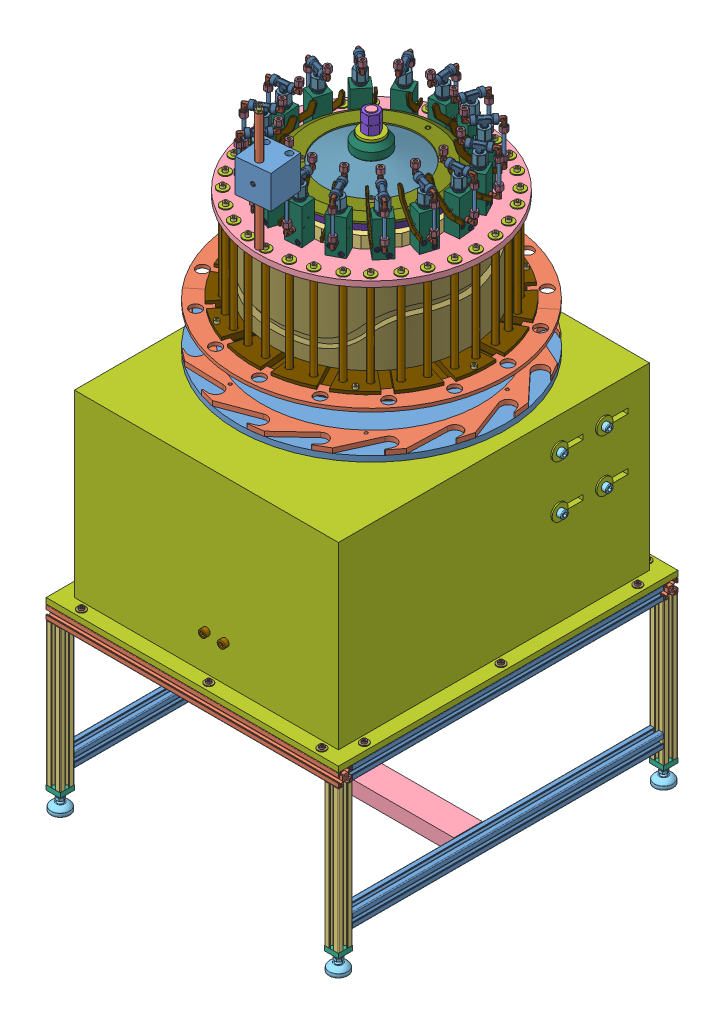
SolidWorks assembly Assieme_FINALE, configuration Default. Lengths in mm. (continued)
Components (placement in the parent): (continued)
- assieme parte rotante-2: assieme parte rotante [Default] at (-79.201 623.9178 -645.7922) x (0 1 0) z (-0.73003 0 0.683415) size (749.63 778.63 778.63) (continued)
  - asta scorrimento carello-18: asta scorrimento carello [Default] at (287.5433 -61.3104 206.5173) x (0 -0.130526 -0.991445) z (-1 0 0) size (12 12 225)
  - asta scorrimento carello-19: asta scorrimento carello [Default] at (287.5433 -135.0285 252.8771) x (0 -0.5 -0.866025) z (-1 0 0) size (12 12 225)
  - asta scorrimento carello-20: asta scorrimento carello [Default] at (287.5433 -185.3939 323.9186) x (0 -0.793353 -0.608761) z (-1 0 0) size (12 12 225)
  - asta scorrimento carello-21: asta scorrimento carello [Default] at (287.5433 -204.7392 408.8264) x (0 -0.965926 -0.258819) z (-1 0 0) size (12 12 225)
  - asta scorrimento carello-22: asta scorrimento carello [Default] at (287.5433 -190.119 494.6741) x (0 -0.991445 0.130526) z (-1 0 0) size (12 12 225)
  - asta scorrimento carello-23: asta scorrimento carello [Default] at (287.5433 -143.7592 568.3922) x (0 -0.866025 0.5) z (-1 0 0) size (12 12 225)
  - asta scorrimento carello-24: asta scorrimento carello [Default] at (287.5433 -72.7177 618.7576) x (0 -0.608761 0.793353) z (-1 0 0) size (12 12 225)
  - asta scorrimento carello-25: asta scorrimento carello [Default] at (287.5433 12.1901 638.1029) x (0 -0.258819 0.965926) z (-1 0 0) size (12 12 225)
  - asta scorrimento carello-26: asta scorrimento carello [Default] at (287.5433 98.0378 623.4827) x (0 0.130526 0.991445) z (-1 0 0) size (12 12 225)
  - asta scorrimento carello-27: asta scorrimento carello [Default] at (287.5433 171.7559 577.1229) x (0 0.5 0.866025) z (-1 0 0) size (12 12 225)
  - asta scorrimento carello-28: asta scorrimento carello [Default] at (287.5433 222.1213 506.0814) x (0 0.793353 0.608761) z (-1 0 0) size (12 12 225)
  - asta scorrimento carello-29: asta scorrimento carello [Default] at (287.5433 241.4666 421.1736) x (0 0.965926 0.258819) z (-1 0 0) size (12 12 225)
  - asta scorrimento carello-30: asta scorrimento carello [Default] at (287.5433 226.8464 335.3259) x (0 0.991445 -0.130526) z (-1 0 0) size (12 12 225)
  - asta scorrimento carello-31: asta scorrimento carello [Default] at (287.5433 180.4866 261.6078) x (0 0.866025 -0.5) z (-1 0 0) size (12 12 225)
  - asta scorrimento carello-32: asta scorrimento carello [Default] at (287.5433 109.4451 211.2424) x (0 0.608761 -0.793353) z (-1 0 0) size (12 12 225)
  - rondella M6-129: rondella M6 [Washer ISO 7094 - 6] at (400.0433 -61.3104 206.5173) x (-1 0 0) z (0 0.991445 -0.130526) size (2 22 22)
  - rondella M6-130: rondella M6 [Washer ISO 7094 - 6] at (400.0433 -135.0285 252.8771) x (-1 0 0) z (0 0.866025 -0.5) size (2 22 22)
  - rondella M6-131: rondella M6 [Washer ISO 7094 - 6] at (400.0433 -185.3939 323.9186) x (-1 0 0) z (0 0.608761 -0.793353) size (2 22 22)
  - rondella M6-132: rondella M6 [Washer ISO 7094 - 6] at (400.0433 -204.7392 408.8264) x (-1 0 0) z (0 0.258819 -0.965926) size (2 22 22)
  - rondella M6-133: rondella M6 [Washer ISO 7094 - 6] at (400.0433 -190.119 494.6741) x (-1 0 0) z (0 -0.130526 -0.991445) size (2 22 22)
  - rondella M6-134: rondella M6 [Washer ISO 7094 - 6] at (400.0433 -143.7592 568.3922) x (-1 0 0) z (0 -0.5 -0.866025) size (2 22 22)
  - rondella M6-135: rondella M6 [Washer ISO 7094 - 6] at (400.0433 -72.7177 618.7576) x (-1 0 0) z (0 -0.793353 -0.608761) size (2 22 22)
  - rondella M6-136: rondella M6 [Washer ISO 7094 - 6] at (400.0433 12.1901 638.1029) x (-1 0 0) z (0 -0.965926 -0.258819) size (2 22 22)
  - rondella M6-137: rondella M6 [Washer ISO 7094 - 6] at (400.0433 98.0378 623.4827) x (-1 0 0) z (0 -0.991445 0.130526) size (2 22 22)
  - rondella M6-138: rondella M6 [Washer ISO 7094 - 6] at (400.0433 171.7559 577.1229) x (-1 0 0) z (0 -0.866025 0.5) size (2 22 22)
  - rondella M6-139: rondella M6 [Washer ISO 7094 - 6] at (400.0433 222.1213 506.0814) x (-1 0 0) z (0 -0.608761 0.793353) size (2 22 22)
  - rondella M6-140: rondella M6 [Washer ISO 7094 - 6] at (400.0433 241.4666 421.1736) x (-1 0 0) z (0 -0.258819 0.965926) size (2 22 22)
  - rondella M6-141: rondella M6 [Washer ISO 7094 - 6] at (400.0433 226.8464 335.3259) x (-1 0 0) z (0 0.130526 0.991445) size (2 22 22)
  - rondella M6-142: rondella M6 [Washer ISO 7094 - 6] at (400.0433 180.4866 261.6078) x (-1 0 0) z (0 0.5 0.866025) size (2 22 22)
  - rondella M6-143: rondella M6 [Washer ISO 7094 - 6] at (400.0433 109.4451 211.2424) x (-1 0 0) z (0 0.793353 0.608761) size (2 22 22)
  - M6 16mm-50: M6 16mm [ISO 4762 M6 x 16 - 16N] at (408.0433 -61.3104 206.5173) x (-1 0 0) z (0 0.130526 0.991445) size (22 10 10)
  - M6 16mm-51: M6 16mm [ISO 4762 M6 x 16 - 16N] at (408.0433 -135.0285 252.8771) x (-1 0 0) z (0 0.5 0.866025) size (22 10 10)
  - M6 16mm-52: M6 16mm [ISO 4762 M6 x 16 - 16N] at (408.0433 -185.3939 323.9186) x (-1 0 0) z (0 0.793353 0.608761) size (22 10 10)
  - M6 16mm-53: M6 16mm [ISO 4762 M6 x 16 - 16N] at (408.0433 -204.7392 408.8264) x (-1 0 0) z (0 0.965926 0.258819) size (22 10 10)
  - M6 16mm-54: M6 16mm [ISO 4762 M6 x 16 - 16N] at (408.0433 -190.119 494.6741) x (-1 0 0) z (0 0.991445 -0.130526) size (22 10 10)
  - M6 16mm-55: M6 16mm [ISO 4762 M6 x 16 - 16N] at (408.0433 -143.7592 568.3922) x (-1 0 0) z (0 0.866025 -0.5) size (22 10 10)
  - M6 16mm-56: M6 16mm [ISO 4762 M6 x 16 - 16N] at (408.0433 -72.7177 618.7576) x (-1 0 0) z (0 0.608761 -0.793353) size (22 10 10)
  - M6 16mm-57: M6 16mm [ISO 4762 M6 x 16 - 16N] at (408.0433 12.1901 638.1029) x (-1 0 0) z (0 0.258819 -0.965926) size (22 10 10)
  - M6 16mm-58: M6 16mm [ISO 4762 M6 x 16 - 16N] at (408.0433 98.0378 623.4827) x (-1 0 0) z (0 -0.130526 -0.991445) size (22 10 10)
  - M6 16mm-59: M6 16mm [ISO 4762 M6 x 16 - 16N] at (408.0433 171.7559 577.1229) x (-1 0 0) z (0 -0.5 -0.866025) size (22 10 10)
  - M6 16mm-60: M6 16mm [ISO 4762 M6 x 16 - 16N] at (408.0433 222.1213 506.0814) x (-1 0 0) z (0 -0.793353 -0.608761) size (22 10 10)
  - M6 16mm-61: M6 16mm [ISO 4762 M6 x 16 - 16N] at (408.0433 241.4666 421.1736) x (-1 0 0) z (0 -0.965926 -0.258819) size (22 10 10)
  - M6 16mm-62: M6 16mm [ISO 4762 M6 x 16 - 16N] at (408.0433 226.8464 335.3259) x (-1 0 0) z (0 -0.991445 0.130526) size (22 10 10)
  - M6 16mm-63: M6 16mm [ISO 4762 M6 x 16 - 16N] at (408.0433 180.4866 261.6078) x (-1 0 0) z (0 -0.866025 0.5) size (22 10 10)
  - M6 16mm-64: M6 16mm [ISO 4762 M6 x 16 - 16N] at (408.0433 109.4451 211.2424) x (-1 0 0) z (0 -0.608761 0.793353) size (22 10 10)
  - AssiemeValvola-2: AssiemeValvola [Default] at (515.3257 40.5532 246.4544) x (0 -0.130526 0.991445) z (0 0.991445 0.130526) size (90.26 138.63 38)
    - RaccordoT-1: RaccordoT [Default] at origin size (43 29.75 16.5)
    - Raccordo a L-1: Raccordo a L [Default] at (-30 0 0) x (0 -1 0) z (0 0 -1) size (28.34 25.51 14.01)
      - 1809_06_10_01-1: 1809_06_10_01 [Default] at origin size (22.49 23 10)
      - 1809_06_10_02-1: 1809_06_10_02 [Default] at origin size (6.5 8.5 8.5)
      - 1809_06_10_03-1: 1809_06_10_03 [Default] at origin size (11.02 15.01 14.01)
    - Raccordo a L-2: Raccordo a L [Default] at (30 0 0) x (0 1 0) z (0 0 -1) size (28.34 25.51 14.01)
      - 1809_06_10_01-1: 1809_06_10_01 [Default] at origin size (22.49 23 10)
      - 1809_06_10_02-1: 1809_06_10_02 [Default] at origin size (6.5 8.5 8.5)
      - 1809_06_10_03-1: 1809_06_10_03 [Default] at origin size (11.02 15.01 14.01)
    - TappoChiusura-1: TappoChiusura [Default] at (0 -32 0) x (0 -1 0) z (0 0 1) size (38.28 26.74 26.74)
    - CorpoValvola-1: CorpoValvola [Default] at (-15 -115.2824 0) size (30 75 34)
    - Raccordo a L-3: Raccordo a L [Default] at (-30 -88.2824 0) x (0 1 0) z (0 0 1) size (28.34 25.51 14.01)
      - 1809_06_10_01-1: 1809_06_10_01 [Default] at origin size (22.49 23 10)
      - 1809_06_10_02-1: 1809_06_10_02 [Default] at origin size (6.5 8.5 8.5)
      - 1809_06_10_03-1: 1809_06_10_03 [Default] at origin size (11.02 15.01 14.01)
    - Spina_3x38-1: Spina_3x38 [Default] at (0 -68.2824 -21) x (-1 0 0) z (0 0 1) size (3 3 38)
    - Spina_3x38-2: Spina_3x38 [Default] at (-10 -80.2824 -21) x (0.996193 0.087174 0) z (0 0 1) size (3 3 38)
    - M5 40mm-3: M5 40mm [ISO 4762 M5 x 40 - 40N] at (-14.6 -108.7824 9) size (45 8.5 8.5)
    - M5 40mm-2: M5 40mm [ISO 4762 M5 x 40 - 40N] at (-14.6 -96.7824 -9) size (45 8.5 8.5)
    - LevaValvola-1: LevaValvola [Default] at (-24.507 -86.571 -17) x (0.996193 0.087174 0) z (0 0 1) size (77.55 60.2 4)
    - Tubo-1: Tubo [Default] at (-30 -15.9665 0) x (1 0 0) z (0 -1 0) size (6 6 56.4)
  - AssiemeValvola-3: AssiemeValvola [Default] at (515.3257 -25.6355 250.7926) x (0 0.258819 0.965926) z (0 0.965926 -0.258819) size (90.26 138.63 38)
    - RaccordoT-1: RaccordoT [Default] at origin size (43 29.75 16.5)
    - Raccordo a L-1: Raccordo a L [Default] at (-30 0 0) x (0 -1 0) z (0 0 -1) size (28.34 25.51 14.01)
      - 1809_06_10_01-1: 1809_06_10_01 [Default] at origin size (22.49 23 10)
      - 1809_06_10_02-1: 1809_06_10_02 [Default] at origin size (6.5 8.5 8.5)
      - 1809_06_10_03-1: 1809_06_10_03 [Default] at origin size (11.02 15.01 14.01)
    - Raccordo a L-2: Raccordo a L [Default] at (30 0 0) x (0 1 0) z (0 0 -1) size (28.34 25.51 14.01)
      - 1809_06_10_01-1: 1809_06_10_01 [Default] at origin size (22.49 23 10)
      - 1809_06_10_02-1: 1809_06_10_02 [Default] at origin size (6.5 8.5 8.5)
      - 1809_06_10_03-1: 1809_06_10_03 [Default] at origin size (11.02 15.01 14.01)
    - TappoChiusura-1: TappoChiusura [Default] at (0 -32 0) x (0 -1 0) z (0 0 1) size (38.28 26.74 26.74)
    - CorpoValvola-1: CorpoValvola [Default] at (-15 -115.2824 0) size (30 75 34)
    - Raccordo a L-3: Raccordo a L [Default] at (-30 -88.2824 0) x (0 1 0) z (0 0 1) size (28.34 25.51 14.01)
      - 1809_06_10_01-1: 1809_06_10_01 [Default] at origin size (22.49 23 10)
      - 1809_06_10_02-1: 1809_06_10_02 [Default] at origin size (6.5 8.5 8.5)
      - 1809_06_10_03-1: 1809_06_10_03 [Default] at origin size (11.02 15.01 14.01)
    - Spina_3x38-1: Spina_3x38 [Default] at (0 -68.2824 -21) x (-1 0 0) z (0 0 1) size (3 3 38)
    - Spina_3x38-2: Spina_3x38 [Default] at (-10 -80.2824 -21) x (0.996193 0.087174 0) z (0 0 1) size (3 3 38)
    - M5 40mm-3: M5 40mm [ISO 4762 M5 x 40 - 40N] at (-14.6 -108.7824 9) size (45 8.5 8.5)
    - M5 40mm-2: M5 40mm [ISO 4762 M5 x 40 - 40N] at (-14.6 -96.7824 -9) size (45 8.5 8.5)
    - LevaValvola-1: LevaValvola [Default] at (-24.507 -86.571 -17) x (0.996193 0.087174 0) z (0 0 1) size (77.55 60.2 4)
    - Tubo-1: Tubo [Default] at (-30 -15.9665 0) x (1 0 0) z (0 -1 0) size (6 6 56.4)
  - AssiemeValvola-4: AssiemeValvola [Default] at (515.3257 -85.1257 280.1299) x (0 0.608761 0.793353) z (0 0.793353 -0.608761) size (90.26 138.63 38)
    - RaccordoT-1: RaccordoT [Default] at origin size (43 29.75 16.5)
    - Raccordo a L-1: Raccordo a L [Default] at (-30 0 0) x (0 -1 0) z (0 0 -1) size (28.34 25.51 14.01)
      - 1809_06_10_01-1: 1809_06_10_01 [Default] at origin size (22.49 23 10)
      - 1809_06_10_02-1: 1809_06_10_02 [Default] at origin size (6.5 8.5 8.5)
      - 1809_06_10_03-1: 1809_06_10_03 [Default] at origin size (11.02 15.01 14.01)
    - Raccordo a L-2: Raccordo a L [Default] at (30 0 0) x (0 1 0) z (0 0 -1) size (28.34 25.51 14.01)
      - 1809_06_10_01-1: 1809_06_10_01 [Default] at origin size (22.49 23 10)
      - 1809_06_10_02-1: 1809_06_10_02 [Default] at origin size (6.5 8.5 8.5)
      - 1809_06_10_03-1: 1809_06_10_03 [Default] at origin size (11.02 15.01 14.01)
    - TappoChiusura-1: TappoChiusura [Default] at (0 -32 0) x (0 -1 0) z (0 0 1) size (38.28 26.74 26.74)
    - CorpoValvola-1: CorpoValvola [Default] at (-15 -115.2824 0) size (30 75 34)
    - Raccordo a L-3: Raccordo a L [Default] at (-30 -88.2824 0) x (0 1 0) z (0 0 1) size (28.34 25.51 14.01)
      - 1809_06_10_01-1: 1809_06_10_01 [Default] at origin size (22.49 23 10)
      - 1809_06_10_02-1: 1809_06_10_02 [Default] at origin size (6.5 8.5 8.5)
      - 1809_06_10_03-1: 1809_06_10_03 [Default] at origin size (11.02 15.01 14.01)
    - Spina_3x38-1: Spina_3x38 [Default] at (0 -68.2824 -21) x (-1 0 0) z (0 0 1) size (3 3 38)
    - Spina_3x38-2: Spina_3x38 [Default] at (-10 -80.2824 -21) x (0.996193 0.087174 0) z (0 0 1) size (3 3 38)
    - M5 40mm-3: M5 40mm [ISO 4762 M5 x 40 - 40N] at (-14.6 -108.7824 9) size (45 8.5 8.5)
    - M5 40mm-2: M5 40mm [ISO 4762 M5 x 40 - 40N] at (-14.6 -96.7824 -9) size (45 8.5 8.5)
    - LevaValvola-1: LevaValvola [Default] at (-24.507 -86.571 -17) x (0.996193 0.087174 0) z (0 0 1) size (77.55 60.2 4)
    - Tubo-1: Tubo [Default] at (-30 -15.9665 0) x (1 0 0) z (0 -1 0) size (6 6 56.4)
  - AssiemeValvola-5: AssiemeValvola [Default] at (515.3257 -128.8606 330) x (0 0.866025 0.5) z (0 0.5 -0.866025) size (90.26 138.63 38)
    - RaccordoT-1: RaccordoT [Default] at origin size (43 29.75 16.5)
    - Raccordo a L-1: Raccordo a L [Default] at (-30 0 0) x (0 -1 0) z (0 0 -1) size (28.34 25.51 14.01)
      - 1809_06_10_01-1: 1809_06_10_01 [Default] at origin size (22.49 23 10)
      - 1809_06_10_02-1: 1809_06_10_02 [Default] at origin size (6.5 8.5 8.5)
      - 1809_06_10_03-1: 1809_06_10_03 [Default] at origin size (11.02 15.01 14.01)
    - Raccordo a L-2: Raccordo a L [Default] at (30 0 0) x (0 1 0) z (0 0 -1) size (28.34 25.51 14.01)
      - 1809_06_10_01-1: 1809_06_10_01 [Default] at origin size (22.49 23 10)
      - 1809_06_10_02-1: 1809_06_10_02 [Default] at origin size (6.5 8.5 8.5)
      - 1809_06_10_03-1: 1809_06_10_03 [Default] at origin size (11.02 15.01 14.01)
    - TappoChiusura-1: TappoChiusura [Default] at (0 -32 0) x (0 -1 0) z (0 0 1) size (38.28 26.74 26.74)
    - CorpoValvola-1: CorpoValvola [Default] at (-15 -115.2824 0) size (30 75 34)
    - Raccordo a L-3: Raccordo a L [Default] at (-30 -88.2824 0) x (0 1 0) z (0 0 1) size (28.34 25.51 14.01)
      - 1809_06_10_01-1: 1809_06_10_01 [Default] at origin size (22.49 23 10)
      - 1809_06_10_02-1: 1809_06_10_02 [Default] at origin size (6.5 8.5 8.5)
      - 1809_06_10_03-1: 1809_06_10_03 [Default] at origin size (11.02 15.01 14.01)
    - Spina_3x38-1: Spina_3x38 [Default] at (0 -68.2824 -21) x (-1 0 0) z (0 0 1) size (3 3 38)
    - Spina_3x38-2: Spina_3x38 [Default] at (-10 -80.2824 -21) x (0.996193 0.087174 0) z (0 0 1) size (3 3 38)
    - M5 40mm-3: M5 40mm [ISO 4762 M5 x 40 - 40N] at (-14.6 -108.7824 9) size (45 8.5 8.5)
    - M5 40mm-2: M5 40mm [ISO 4762 M5 x 40 - 40N] at (-14.6 -96.7824 -9) size (45 8.5 8.5)
    - LevaValvola-1: LevaValvola [Default] at (-24.507 -86.571 -17) x (0.996193 0.087174 0) z (0 0 1) size (77.55 60.2 4)
    - Tubo-1: Tubo [Default] at (-30 -15.9665 0) x (1 0 0) z (0 -1 0) size (6 6 56.4)
  - AssiemeValvola-6: AssiemeValvola [Default] at (515.3257 -150.1819 392.8105) x (0 0.991445 0.130526) z (0 0.130526 -0.991445) size (90.26 138.63 38)
    - RaccordoT-1: RaccordoT [Default] at origin size (43 29.75 16.5)
    - Raccordo a L-1: Raccordo a L [Default] at (-30 0 0) x (0 -1 0) z (0 0 -1) size (28.34 25.51 14.01)
      - 1809_06_10_01-1: 1809_06_10_01 [Default] at origin size (22.49 23 10)
      - 1809_06_10_02-1: 1809_06_10_02 [Default] at origin size (6.5 8.5 8.5)
      - 1809_06_10_03-1: 1809_06_10_03 [Default] at origin size (11.02 15.01 14.01)
    - Raccordo a L-2: Raccordo a L [Default] at (30 0 0) x (0 1 0) z (0 0 -1) size (28.34 25.51 14.01)
      - 1809_06_10_01-1: 1809_06_10_01 [Default] at origin size (22.49 23 10)
      - 1809_06_10_02-1: 1809_06_10_02 [Default] at origin size (6.5 8.5 8.5)
      - 1809_06_10_03-1: 1809_06_10_03 [Default] at origin size (11.02 15.01 14.01)
    - TappoChiusura-1: TappoChiusura [Default] at (0 -32 0) x (0 -1 0) z (0 0 1) size (38.28 26.74 26.74)
    - CorpoValvola-1: CorpoValvola [Default] at (-15 -115.2824 0) size (30 75 34)
    - Raccordo a L-3: Raccordo a L [Default] at (-30 -88.2824 0) x (0 1 0) z (0 0 1) size (28.34 25.51 14.01)
      - 1809_06_10_01-1: 1809_06_10_01 [Default] at origin size (22.49 23 10)
      - 1809_06_10_02-1: 1809_06_10_02 [Default] at origin size (6.5 8.5 8.5)
      - 1809_06_10_03-1: 1809_06_10_03 [Default] at origin size (11.02 15.01 14.01)
    - Spina_3x38-1: Spina_3x38 [Default] at (0 -68.2824 -21) x (-1 0 0) z (0 0 1) size (3 3 38)
    - Spina_3x38-2: Spina_3x38 [Default] at (-10 -80.2824 -21) x (0.996193 0.087174 0) z (0 0 1) size (3 3 38)
    - M5 40mm-3: M5 40mm [ISO 4762 M5 x 40 - 40N] at (-14.6 -108.7824 9) size (45 8.5 8.5)
    - M5 40mm-2: M5 40mm [ISO 4762 M5 x 40 - 40N] at (-14.6 -96.7824 -9) size (45 8.5 8.5)
    - LevaValvola-1: LevaValvola [Default] at (-24.507 -86.571 -17) x (0.996193 0.087174 0) z (0 0 1) size (77.55 60.2 4)
    - Tubo-1: Tubo [Default] at (-30 -15.9665 0) x (1 0 0) z (0 -1 0) size (6 6 56.4)
  - AssiemeValvola-7: AssiemeValvola [Default] at (515.3257 -145.8437 458.9992) x (0 0.965926 -0.258819) z (0 -0.258819 -0.965926) size (90.26 138.63 38)
    - RaccordoT-1: RaccordoT [Default] at origin size (43 29.75 16.5)
    - Raccordo a L-1: Raccordo a L [Default] at (-30 0 0) x (0 -1 0) z (0 0 -1) size (28.34 25.51 14.01)
      - 1809_06_10_01-1: 1809_06_10_01 [Default] at origin size (22.49 23 10)
      - 1809_06_10_02-1: 1809_06_10_02 [Default] at origin size (6.5 8.5 8.5)
      - 1809_06_10_03-1: 1809_06_10_03 [Default] at origin size (11.02 15.01 14.01)
    - Raccordo a L-2: Raccordo a L [Default] at (30 0 0) x (0 1 0) z (0 0 -1) size (28.34 25.51 14.01)
      - 1809_06_10_01-1: 1809_06_10_01 [Default] at origin size (22.49 23 10)
      - 1809_06_10_02-1: 1809_06_10_02 [Default] at origin size (6.5 8.5 8.5)
      - 1809_06_10_03-1: 1809_06_10_03 [Default] at origin size (11.02 15.01 14.01)
    - TappoChiusura-1: TappoChiusura [Default] at (0 -32 0) x (0 -1 0) z (0 0 1) size (38.28 26.74 26.74)
    - CorpoValvola-1: CorpoValvola [Default] at (-15 -115.2824 0) size (30 75 34)
    - Raccordo a L-3: Raccordo a L [Default] at (-30 -88.2824 0) x (0 1 0) z (0 0 1) size (28.34 25.51 14.01)
      - 1809_06_10_01-1: 1809_06_10_01 [Default] at origin size (22.49 23 10)
      - 1809_06_10_02-1: 1809_06_10_02 [Default] at origin size (6.5 8.5 8.5)
      - 1809_06_10_03-1: 1809_06_10_03 [Default] at origin size (11.02 15.01 14.01)
    - Spina_3x38-1: Spina_3x38 [Default] at (0 -68.2824 -21) x (-1 0 0) z (0 0 1) size (3 3 38)
    - Spina_3x38-2: Spina_3x38 [Default] at (-10 -80.2824 -21) x (0.996193 0.087174 0) z (0 0 1) size (3 3 38)
    - M5 40mm-3: M5 40mm [ISO 4762 M5 x 40 - 40N] at (-14.6 -108.7824 9) size (45 8.5 8.5)
    - M5 40mm-2: M5 40mm [ISO 4762 M5 x 40 - 40N] at (-14.6 -96.7824 -9) size (45 8.5 8.5)
    - LevaValvola-1: LevaValvola [Default] at (-24.507 -86.571 -17) x (0.996193 0.087174 0) z (0 0 1) size (77.55 60.2 4)
    - Tubo-1: Tubo [Default] at (-30 -15.9665 0) x (1 0 0) z (0 -1 0) size (6 6 56.4)
  - AssiemeValvola-8: AssiemeValvola [Default] at (515.3257 -116.5064 518.4894) x (0 0.793353 -0.608761) z (0 -0.608761 -0.793353) size (90.26 138.63 38)
    - RaccordoT-1: RaccordoT [Default] at origin size (43 29.75 16.5)
    - Raccordo a L-1: Raccordo a L [Default] at (-30 0 0) x (0 -1 0) z (0 0 -1) size (28.34 25.51 14.01)
      - 1809_06_10_01-1: 1809_06_10_01 [Default] at origin size (22.49 23 10)
      - 1809_06_10_02-1: 1809_06_10_02 [Default] at origin size (6.5 8.5 8.5)
      - 1809_06_10_03-1: 1809_06_10_03 [Default] at origin size (11.02 15.01 14.01)
    - Raccordo a L-2: Raccordo a L [Default] at (30 0 0) x (0 1 0) z (0 0 -1) size (28.34 25.51 14.01)
      - 1809_06_10_01-1: 1809_06_10_01 [Default] at origin size (22.49 23 10)
      - 1809_06_10_02-1: 1809_06_10_02 [Default] at origin size (6.5 8.5 8.5)
      - 1809_06_10_03-1: 1809_06_10_03 [Default] at origin size (11.02 15.01 14.01)
    - TappoChiusura-1: TappoChiusura [Default] at (0 -32 0) x (0 -1 0) z (0 0 1) size (38.28 26.74 26.74)
    - CorpoValvola-1: CorpoValvola [Default] at (-15 -115.2824 0) size (30 75 34)
    - Raccordo a L-3: Raccordo a L [Default] at (-30 -88.2824 0) x (0 1 0) z (0 0 1) size (28.34 25.51 14.01)
      - 1809_06_10_01-1: 1809_06_10_01 [Default] at origin size (22.49 23 10)
      - 1809_06_10_02-1: 1809_06_10_02 [Default] at origin size (6.5 8.5 8.5)
      - 1809_06_10_03-1: 1809_06_10_03 [Default] at origin size (11.02 15.01 14.01)
    - Spina_3x38-1: Spina_3x38 [Default] at (0 -68.2824 -21) x (-1 0 0) z (0 0 1) size (3 3 38)
    - Spina_3x38-2: Spina_3x38 [Default] at (-10 -80.2824 -21) x (0.996193 0.087174 0) z (0 0 1) size (3 3 38)
    - M5 40mm-3: M5 40mm [ISO 4762 M5 x 40 - 40N] at (-14.6 -108.7824 9) size (45 8.5 8.5)
    - M5 40mm-2: M5 40mm [ISO 4762 M5 x 40 - 40N] at (-14.6 -96.7824 -9) size (45 8.5 8.5)
    - LevaValvola-1: LevaValvola [Default] at (-24.507 -86.571 -17) x (0.996193 0.087174 0) z (0 0 1) size (77.55 60.2 4)
    - Tubo-1: Tubo [Default] at (-30 -15.9665 0) x (1 0 0) z (0 -1 0) size (6 6 56.4)
  - AssiemeValvola-9: AssiemeValvola [Default] at (515.3257 -66.6363 562.2243) x (0 0.5 -0.866025) z (0 -0.866025 -0.5) size (90.26 138.63 38)
    - RaccordoT-1: RaccordoT [Default] at origin size (43 29.75 16.5)
    - Raccordo a L-1: Raccordo a L [Default] at (-30 0 0) x (0 -1 0) z (0 0 -1) size (28.34 25.51 14.01)
      - 1809_06_10_01-1: 1809_06_10_01 [Default] at origin size (22.49 23 10)
      - 1809_06_10_02-1: 1809_06_10_02 [Default] at origin size (6.5 8.5 8.5)
      - 1809_06_10_03-1: 1809_06_10_03 [Default] at origin size (11.02 15.01 14.01)
    - Raccordo a L-2: Raccordo a L [Default] at (30 0 0) x (0 1 0) z (0 0 -1) size (28.34 25.51 14.01)
      - 1809_06_10_01-1: 1809_06_10_01 [Default] at origin size (22.49 23 10)
      - 1809_06_10_02-1: 1809_06_10_02 [Default] at origin size (6.5 8.5 8.5)
      - 1809_06_10_03-1: 1809_06_10_03 [Default] at origin size (11.02 15.01 14.01)
    - TappoChiusura-1: TappoChiusura [Default] at (0 -32 0) x (0 -1 0) z (0 0 1) size (38.28 26.74 26.74)
    - CorpoValvola-1: CorpoValvola [Default] at (-15 -115.2824 0) size (30 75 34)
    - Raccordo a L-3: Raccordo a L [Default] at (-30 -88.2824 0) x (0 1 0) z (0 0 1) size (28.34 25.51 14.01)
      - 1809_06_10_01-1: 1809_06_10_01 [Default] at origin size (22.49 23 10)
      - 1809_06_10_02-1: 1809_06_10_02 [Default] at origin size (6.5 8.5 8.5)
      - 1809_06_10_03-1: 1809_06_10_03 [Default] at origin size (11.02 15.01 14.01)
    - Spina_3x38-1: Spina_3x38 [Default] at (0 -68.2824 -21) x (-1 0 0) z (0 0 1) size (3 3 38)
    - Spina_3x38-2: Spina_3x38 [Default] at (-10 -80.2824 -21) x (0.996193 0.087174 0) z (0 0 1) size (3 3 38)
    - M5 40mm-3: M5 40mm [ISO 4762 M5 x 40 - 40N] at (-14.6 -108.7824 9) size (45 8.5 8.5)
    - M5 40mm-2: M5 40mm [ISO 4762 M5 x 40 - 40N] at (-14.6 -96.7824 -9) size (45 8.5 8.5)
    - LevaValvola-1: LevaValvola [Default] at (-24.507 -86.571 -17) x (0.996193 0.087174 0) z (0 0 1) size (77.55 60.2 4)
    - Tubo-1: Tubo [Default] at (-30 -15.9665 0) x (1 0 0) z (0 -1 0) size (6 6 56.4)
  - AssiemeValvola-10: AssiemeValvola [Default] at (515.3257 -3.8258 583.5456) x (0 0.130526 -0.991445) z (0 -0.991445 -0.130526) size (90.26 138.63 38)
    - RaccordoT-1: RaccordoT [Default] at origin size (43 29.75 16.5)
    - Raccordo a L-1: Raccordo a L [Default] at (-30 0 0) x (0 -1 0) z (0 0 -1) size (28.34 25.51 14.01)
      - 1809_06_10_01-1: 1809_06_10_01 [Default] at origin size (22.49 23 10)
      - 1809_06_10_02-1: 1809_06_10_02 [Default] at origin size (6.5 8.5 8.5)
      - 1809_06_10_03-1: 1809_06_10_03 [Default] at origin size (11.02 15.01 14.01)
    - Raccordo a L-2: Raccordo a L [Default] at (30 0 0) x (0 1 0) z (0 0 -1) size (28.34 25.51 14.01)
      - 1809_06_10_01-1: 1809_06_10_01 [Default] at origin size (22.49 23 10)
      - 1809_06_10_02-1: 1809_06_10_02 [Default] at origin size (6.5 8.5 8.5)
      - 1809_06_10_03-1: 1809_06_10_03 [Default] at origin size (11.02 15.01 14.01)
    - TappoChiusura-1: TappoChiusura [Default] at (0 -32 0) x (0 -1 0) z (0 0 1) size (38.28 26.74 26.74)
    - CorpoValvola-1: CorpoValvola [Default] at (-15 -115.2824 0) size (30 75 34)
    - Raccordo a L-3: Raccordo a L [Default] at (-30 -88.2824 0) x (0 1 0) z (0 0 1) size (28.34 25.51 14.01)
      - 1809_06_10_01-1: 1809_06_10_01 [Default] at origin size (22.49 23 10)
      - 1809_06_10_02-1: 1809_06_10_02 [Default] at origin size (6.5 8.5 8.5)
      - 1809_06_10_03-1: 1809_06_10_03 [Default] at origin size (11.02 15.01 14.01)
    - Spina_3x38-1: Spina_3x38 [Default] at (0 -68.2824 -21) x (-1 0 0) z (0 0 1) size (3 3 38)
    - Spina_3x38-2: Spina_3x38 [Default] at (-10 -80.2824 -21) x (0.996193 0.087174 0) z (0 0 1) size (3 3 38)
    - M5 40mm-3: M5 40mm [ISO 4762 M5 x 40 - 40N] at (-14.6 -108.7824 9) size (45 8.5 8.5)
    - M5 40mm-2: M5 40mm [ISO 4762 M5 x 40 - 40N] at (-14.6 -96.7824 -9) size (45 8.5 8.5)
    - LevaValvola-1: LevaValvola [Default] at (-24.507 -86.571 -17) x (0.996193 0.087174 0) z (0 0 1) size (77.55 60.2 4)
    - Tubo-1: Tubo [Default] at (-30 -15.9665 0) x (1 0 0) z (0 -1 0) size (6 6 56.4)
  - AssiemeValvola-11: AssiemeValvola [Default] at (515.3257 62.3629 579.2074) x (0 -0.258819 -0.965926) z (0 -0.965926 0.258819) size (90.26 138.63 38)
    - RaccordoT-1: RaccordoT [Default] at origin size (43 29.75 16.5)
    - Raccordo a L-1: Raccordo a L [Default] at (-30 0 0) x (0 -1 0) z (0 0 -1) size (28.34 25.51 14.01)
      - 1809_06_10_01-1: 1809_06_10_01 [Default] at origin size (22.49 23 10)
      - 1809_06_10_02-1: 1809_06_10_02 [Default] at origin size (6.5 8.5 8.5)
      - 1809_06_10_03-1: 1809_06_10_03 [Default] at origin size (11.02 15.01 14.01)
    - Raccordo a L-2: Raccordo a L [Default] at (30 0 0) x (0 1 0) z (0 0 -1) size (28.34 25.51 14.01)
      - 1809_06_10_01-1: 1809_06_10_01 [Default] at origin size (22.49 23 10)
      - 1809_06_10_02-1: 1809_06_10_02 [Default] at origin size (6.5 8.5 8.5)
      - 1809_06_10_03-1: 1809_06_10_03 [Default] at origin size (11.02 15.01 14.01)
    - TappoChiusura-1: TappoChiusura [Default] at (0 -32 0) x (0 -1 0) z (0 0 1) size (38.28 26.74 26.74)
    - CorpoValvola-1: CorpoValvola [Default] at (-15 -115.2824 0) size (30 75 34)
    - Raccordo a L-3: Raccordo a L [Default] at (-30 -88.2824 0) x (0 1 0) z (0 0 1) size (28.34 25.51 14.01)
      - 1809_06_10_01-1: 1809_06_10_01 [Default] at origin size (22.49 23 10)
      - 1809_06_10_02-1: 1809_06_10_02 [Default] at origin size (6.5 8.5 8.5)
      - 1809_06_10_03-1: 1809_06_10_03 [Default] at origin size (11.02 15.01 14.01)
    - Spina_3x38-1: Spina_3x38 [Default] at (0 -68.2824 -21) x (-1 0 0) z (0 0 1) size (3 3 38)
    - Spina_3x38-2: Spina_3x38 [Default] at (-10 -80.2824 -21) x (0.996193 0.087174 0) z (0 0 1) size (3 3 38)
    - M5 40mm-3: M5 40mm [ISO 4762 M5 x 40 - 40N] at (-14.6 -108.7824 9) size (45 8.5 8.5)
    - M5 40mm-2: M5 40mm [ISO 4762 M5 x 40 - 40N] at (-14.6 -96.7824 -9) size (45 8.5 8.5)
    - LevaValvola-1: LevaValvola [Default] at (-24.507 -86.571 -17) x (0.996193 0.087174 0) z (0 0 1) size (77.55 60.2 4)
    - Tubo-1: Tubo [Default] at (-30 -15.9665 0) x (1 0 0) z (0 -1 0) size (6 6 56.4)
  - AssiemeValvola-12: AssiemeValvola [Default] at (515.3257 121.8531 549.8701) x (0 -0.608761 -0.793353) z (0 -0.793353 0.608761) size (90.26 138.63 38)
    - RaccordoT-1: RaccordoT [Default] at origin size (43 29.75 16.5)
    - Raccordo a L-1: Raccordo a L [Default] at (-30 0 0) x (0 -1 0) z (0 0 -1) size (28.34 25.51 14.01)
      - 1809_06_10_01-1: 1809_06_10_01 [Default] at origin size (22.49 23 10)
      - 1809_06_10_02-1: 1809_06_10_02 [Default] at origin size (6.5 8.5 8.5)
      - 1809_06_10_03-1: 1809_06_10_03 [Default] at origin size (11.02 15.01 14.01)
    - Raccordo a L-2: Raccordo a L [Default] at (30 0 0) x (0 1 0) z (0 0 -1) size (28.34 25.51 14.01)
      - 1809_06_10_01-1: 1809_06_10_01 [Default] at origin size (22.49 23 10)
      - 1809_06_10_02-1: 1809_06_10_02 [Default] at origin size (6.5 8.5 8.5)
      - 1809_06_10_03-1: 1809_06_10_03 [Default] at origin size (11.02 15.01 14.01)
    - TappoChiusura-1: TappoChiusura [Default] at (0 -32 0) x (0 -1 0) z (0 0 1) size (38.28 26.74 26.74)
    - CorpoValvola-1: CorpoValvola [Default] at (-15 -115.2824 0) size (30 75 34)
    - Raccordo a L-3: Raccordo a L [Default] at (-30 -88.2824 0) x (0 1 0) z (0 0 1) size (28.34 25.51 14.01)
      - 1809_06_10_01-1: 1809_06_10_01 [Default] at origin size (22.49 23 10)
      - 1809_06_10_02-1: 1809_06_10_02 [Default] at origin size (6.5 8.5 8.5)
      - 1809_06_10_03-1: 1809_06_10_03 [Default] at origin size (11.02 15.01 14.01)
    - Spina_3x38-1: Spina_3x38 [Default] at (0 -68.2824 -21) x (-1 0 0) z (0 0 1) size (3 3 38)
    - Spina_3x38-2: Spina_3x38 [Default] at (-10 -80.2824 -21) x (0.996193 0.087174 0) z (0 0 1) size (3 3 38)
    - M5 40mm-3: M5 40mm [ISO 4762 M5 x 40 - 40N] at (-14.6 -108.7824 9) size (45 8.5 8.5)
    - M5 40mm-2: M5 40mm [ISO 4762 M5 x 40 - 40N] at (-14.6 -96.7824 -9) size (45 8.5 8.5)
    - LevaValvola-1: LevaValvola [Default] at (-24.507 -86.571 -17) x (0.996193 0.087174 0) z (0 0 1) size (77.55 60.2 4)
    - Tubo-1: Tubo [Default] at (-30 -15.9665 0) x (1 0 0) z (0 -1 0) size (6 6 56.4)
  - AssiemeValvola-13: AssiemeValvola [Default] at (515.3257 165.588 500) x (0 -0.866025 -0.5) z (0 -0.5 0.866025) size (90.26 138.63 38)
    - RaccordoT-1: RaccordoT [Default] at origin size (43 29.75 16.5)
    - Raccordo a L-1: Raccordo a L [Default] at (-30 0 0) x (0 -1 0) z (0 0 -1) size (28.34 25.51 14.01)
      - 1809_06_10_01-1: 1809_06_10_01 [Default] at origin size (22.49 23 10)
      - 1809_06_10_02-1: 1809_06_10_02 [Default] at origin size (6.5 8.5 8.5)
      - 1809_06_10_03-1: 1809_06_10_03 [Default] at origin size (11.02 15.01 14.01)
    - Raccordo a L-2: Raccordo a L [Default] at (30 0 0) x (0 1 0) z (0 0 -1) size (28.34 25.51 14.01)
      - 1809_06_10_01-1: 1809_06_10_01 [Default] at origin size (22.49 23 10)
      - 1809_06_10_02-1: 1809_06_10_02 [Default] at origin size (6.5 8.5 8.5)
      - 1809_06_10_03-1: 1809_06_10_03 [Default] at origin size (11.02 15.01 14.01)
    - TappoChiusura-1: TappoChiusura [Default] at (0 -32 0) x (0 -1 0) z (0 0 1) size (38.28 26.74 26.74)
    - CorpoValvola-1: CorpoValvola [Default] at (-15 -115.2824 0) size (30 75 34)
    - Raccordo a L-3: Raccordo a L [Default] at (-30 -88.2824 0) x (0 1 0) z (0 0 1) size (28.34 25.51 14.01)
      - 1809_06_10_01-1: 1809_06_10_01 [Default] at origin size (22.49 23 10)
      - 1809_06_10_02-1: 1809_06_10_02 [Default] at origin size (6.5 8.5 8.5)
      - 1809_06_10_03-1: 1809_06_10_03 [Default] at origin size (11.02 15.01 14.01)
    - Spina_3x38-1: Spina_3x38 [Default] at (0 -68.2824 -21) x (-1 0 0) z (0 0 1) size (3 3 38)
    - Spina_3x38-2: Spina_3x38 [Default] at (-10 -80.2824 -21) x (0.996193 0.087174 0) z (0 0 1) size (3 3 38)
    - M5 40mm-3: M5 40mm [ISO 4762 M5 x 40 - 40N] at (-14.6 -108.7824 9) size (45 8.5 8.5)
    - M5 40mm-2: M5 40mm [ISO 4762 M5 x 40 - 40N] at (-14.6 -96.7824 -9) size (45 8.5 8.5)
    - LevaValvola-1: LevaValvola [Default] at (-24.507 -86.571 -17) x (0.996193 0.087174 0) z (0 0 1) size (77.55 60.2 4)
    - Tubo-1: Tubo [Default] at (-30 -15.9665 0) x (1 0 0) z (0 -1 0) size (6 6 56.4)
  - AssiemeValvola-14: AssiemeValvola [Default] at (515.3257 186.9093 437.1895) x (0 -0.991445 -0.130526) z (0 -0.130526 0.991445) size (90.26 138.63 38)
    - RaccordoT-1: RaccordoT [Default] at origin size (43 29.75 16.5)
    - Raccordo a L-1: Raccordo a L [Default] at (-30 0 0) x (0 -1 0) z (0 0 -1) size (28.34 25.51 14.01)
      - 1809_06_10_01-1: 1809_06_10_01 [Default] at origin size (22.49 23 10)
      - 1809_06_10_02-1: 1809_06_10_02 [Default] at origin size (6.5 8.5 8.5)
      - 1809_06_10_03-1: 1809_06_10_03 [Default] at origin size (11.02 15.01 14.01)
    - Raccordo a L-2: Raccordo a L [Default] at (30 0 0) x (0 1 0) z (0 0 -1) size (28.34 25.51 14.01)
      - 1809_06_10_01-1: 1809_06_10_01 [Default] at origin size (22.49 23 10)
      - 1809_06_10_02-1: 1809_06_10_02 [Default] at origin size (6.5 8.5 8.5)
      - 1809_06_10_03-1: 1809_06_10_03 [Default] at origin size (11.02 15.01 14.01)
    - TappoChiusura-1: TappoChiusura [Default] at (0 -32 0) x (0 -1 0) z (0 0 1) size (38.28 26.74 26.74)
    - CorpoValvola-1: CorpoValvola [Default] at (-15 -115.2824 0) size (30 75 34)
    - Raccordo a L-3: Raccordo a L [Default] at (-30 -88.2824 0) x (0 1 0) z (0 0 1) size (28.34 25.51 14.01)
      - 1809_06_10_01-1: 1809_06_10_01 [Default] at origin size (22.49 23 10)
      - 1809_06_10_02-1: 1809_06_10_02 [Default] at origin size (6.5 8.5 8.5)
      - 1809_06_10_03-1: 1809_06_10_03 [Default] at origin size (11.02 15.01 14.01)
    - Spina_3x38-1: Spina_3x38 [Default] at (0 -68.2824 -21) x (-1 0 0) z (0 0 1) size (3 3 38)
    - Spina_3x38-2: Spina_3x38 [Default] at (-10 -80.2824 -21) x (0.996193 0.087174 0) z (0 0 1) size (3 3 38)
    - M5 40mm-3: M5 40mm [ISO 4762 M5 x 40 - 40N] at (-14.6 -108.7824 9) size (45 8.5 8.5)
    - M5 40mm-2: M5 40mm [ISO 4762 M5 x 40 - 40N] at (-14.6 -96.7824 -9) size (45 8.5 8.5)
    - LevaValvola-1: LevaValvola [Default] at (-24.507 -86.571 -17) x (0.996193 0.087174 0) z (0 0 1) size (77.55 60.2 4)
    - Tubo-1: Tubo [Default] at (-30 -15.9665 0) x (1 0 0) z (0 -1 0) size (6 6 56.4)
  - AssiemeValvola-15: AssiemeValvola [Default] at (515.3257 182.5711 371.0008) x (0 -0.965926 0.258819) z (0 0.258819 0.965926) size (90.26 138.63 38)
    - RaccordoT-1: RaccordoT [Default] at origin size (43 29.75 16.5)
    - Raccordo a L-1: Raccordo a L [Default] at (-30 0 0) x (0 -1 0) z (0 0 -1) size (28.34 25.51 14.01)
      - 1809_06_10_01-1: 1809_06_10_01 [Default] at origin size (22.49 23 10)
      - 1809_06_10_02-1: 1809_06_10_02 [Default] at origin size (6.5 8.5 8.5)
      - 1809_06_10_03-1: 1809_06_10_03 [Default] at origin size (11.02 15.01 14.01)
    - Raccordo a L-2: Raccordo a L [Default] at (30 0 0) x (0 1 0) z (0 0 -1) size (28.34 25.51 14.01)
      - 1809_06_10_01-1: 1809_06_10_01 [Default] at origin size (22.49 23 10)
      - 1809_06_10_02-1: 1809_06_10_02 [Default] at origin size (6.5 8.5 8.5)
      - 1809_06_10_03-1: 1809_06_10_03 [Default] at origin size (11.02 15.01 14.01)
    - TappoChiusura-1: TappoChiusura [Default] at (0 -32 0) x (0 -1 0) z (0 0 1) size (38.28 26.74 26.74)
    - CorpoValvola-1: CorpoValvola [Default] at (-15 -115.2824 0) size (30 75 34)
    - Raccordo a L-3: Raccordo a L [Default] at (-30 -88.2824 0) x (0 1 0) z (0 0 1) size (28.34 25.51 14.01)
      - 1809_06_10_01-1: 1809_06_10_01 [Default] at origin size (22.49 23 10)
      - 1809_06_10_02-1: 1809_06_10_02 [Default] at origin size (6.5 8.5 8.5)
      - 1809_06_10_03-1: 1809_06_10_03 [Default] at origin size (11.02 15.01 14.01)
    - Spina_3x38-1: Spina_3x38 [Default] at (0 -68.2824 -21) x (-1 0 0) z (0 0 1) size (3 3 38)
    - Spina_3x38-2: Spina_3x38 [Default] at (-10 -80.2824 -21) x (0.996193 0.087174 0) z (0 0 1) size (3 3 38)
    - M5 40mm-3: M5 40mm [ISO 4762 M5 x 40 - 40N] at (-14.6 -108.7824 9) size (45 8.5 8.5)
    - M5 40mm-2: M5 40mm [ISO 4762 M5 x 40 - 40N] at (-14.6 -96.7824 -9) size (45 8.5 8.5)
    - LevaValvola-1: LevaValvola [Default] at (-24.507 -86.571 -17) x (0.996193 0.087174 0) z (0 0 1) size (77.55 60.2 4)
    - Tubo-1: Tubo [Default] at (-30 -15.9665 0) x (1 0 0) z (0 -1 0) size (6 6 56.4)
  - AssiemeValvola-16: AssiemeValvola [Default] at (515.3257 153.2338 311.5106) x (0 -0.793353 0.608761) z (0 0.608761 0.793353) size (90.26 138.63 38)
    - RaccordoT-1: RaccordoT [Default] at origin size (43 29.75 16.5)
    - Raccordo a L-1: Raccordo a L [Default] at (-30 0 0) x (0 -1 0) z (0 0 -1) size (28.34 25.51 14.01)
      - 1809_06_10_01-1: 1809_06_10_01 [Default] at origin size (22.49 23 10)
      - 1809_06_10_02-1: 1809_06_10_02 [Default] at origin size (6.5 8.5 8.5)
      - 1809_06_10_03-1: 1809_06_10_03 [Default] at origin size (11.02 15.01 14.01)
